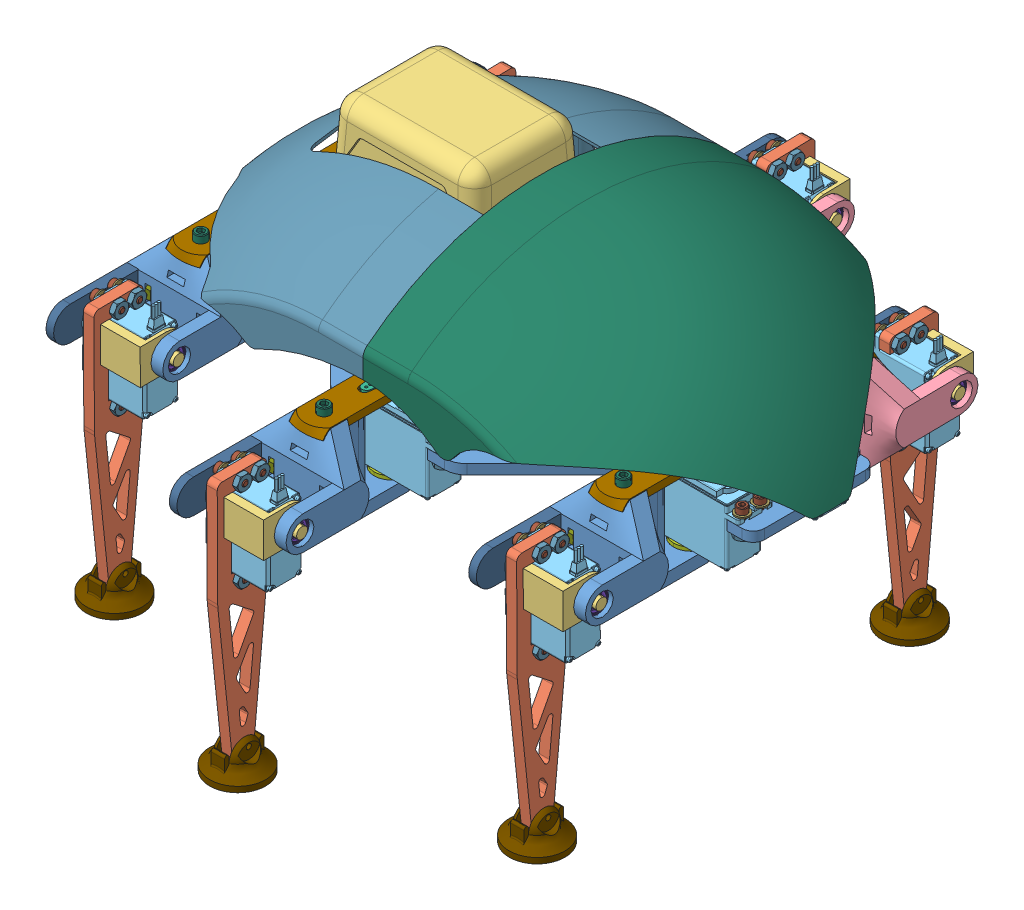
SolidWorks assembly Hexapod_(Leg_V1+Body_V2), configuration Défaut. Lengths in mm.
Overall size (338.69 233.7 350.76).
398 component instances, 33 part files, 150 mates.
Components (placement in the parent):
- Body_V2-5: Body_V2 [Default] at (-310 -5.6 15) x (1 0 0) z (0 1 0) size (310 170 5.6)
- Leg_(Straight_Foot)-6: Leg_(Straight_Foot) [Default] at (-54.94 -26.67 -0.094) size (71.12 162.26 125.96)
  - Foot_(Straight)-1: Foot_(Straight) [Default] at (4.9357 4.6699 -91.3683) x (0.014203 -0.004158 0.99989) z (-0.999899 0 0.014203) size (28 145.4 6)
  - bearing_mount_foot-1: bearing_mount_foot [Default] at (4.8169 16.6428 -99.7277) x (-0.014203 0.004158 -0.99989) z (0.999899 0 -0.014203) size (25 20 29.5)
  - Joint-1: Joint [Défaut] at (35.768 26.4662 -54.7315) x (-0.014203 0 -0.999899) z (0 1 0) size (96.52 53.26 53.26)
  - hs-422-2: hs-422 [Défaut] at (5.1023 6.6131 -77.4551) x (-0.014203 0.004158 -0.99989) z (0.000059 0.999991 0.004158) size (19.81 42.09 58.23)
  - hs-422-3: hs-422 [Défaut] at (19.939 20.701 -19.812) x (0 0 1) z (-1 0 0) size (19.81 42.09 58.23)
  - hs-422_horn_straight-1: hs-422_horn_straight [Default] at (-16.9088 16.9412 -87.0065) x (0.014203 0 0.999899) z (0 1 0) size (33.93 4.93 8.79)
  - hs-422_horn_straight-2: hs-422_horn_straight [Default] at (9.652 42.5743 -9.906) x (-0.014203 0 -0.999899) z (-0.999899 0 0.014203) size (33.93 4.93 8.79)
  - Bearing_mount_leg-1: Bearing_mount_leg [Default] at (9.652 21 2.594) x (0 0 1) z (0 -1 0) size (35 20 30)
  - Bearing-1: Bearing [Default] at (9.652 -6.7498 -9.906) x (0.84763 0 0.530588) z (-0.530588 0 0.84763) size (13.87 4.75 13.87)
  - Bearing-2: Bearing [Default] at (32.2403 16.9412 -87.7047) x (0.007588 -0.845349 0.534161) z (-0.012007 -0.534214 -0.845264) size (13.87 4.75 13.87)
  - Joint_attachment_leg-1: Joint_attachment_leg [Défaut] at (35.768 26.4662 -54.7315) x (-0.014203 0 -0.999899) z (0 1 0) size (74.32 19.07 4.32)
  - Joint_attachment_foot-1: Joint_attachment_foot [Défaut] at (35.768 26.4662 -54.7315) x (-0.014203 0 -0.999899) z (0 1 0) size (64.08 6.7 19.07)
  - socket_1_2_6-32_with_washer-1: socket_1_2_6-32_with_washer [Défaut] at (43.4196 -14.698 -83.8589) x (0.999899 0 -0.014203) z (0.012271 -0.503597 0.863852) size (16.21 7.92 7.92)
    - HX-SHCS 0.138-32x0.5x0.5-N-1: HX-SHCS 0.138-32x0.5x0.5-N [HX-SHCS 0.138-32x0.5x0.5-N] at (-51.206 -1.62 2.0257) size (16.21 5.74 5.74)
    - Narrow FW 0.138-1: Narrow FW 0.138 [Narrow FW 0.138] at (-46.888 -1.62 2.0257) size (0.81 7.92 7.92)
  - socket_1_2_6-32_with_washer-2: socket_1_2_6-32_with_washer [Défaut] at (43.2654 -19.0943 -94.7118) x (0.999899 0 -0.014203) z (0.000059 0.999991 0.004158) size (16.21 7.92 7.92)
    - HX-SHCS 0.138-32x0.5x0.5-N-1: HX-SHCS 0.138-32x0.5x0.5-N [HX-SHCS 0.138-32x0.5x0.5-N] at (-51.206 -1.62 2.0257) size (16.21 5.74 5.74)
    - Narrow FW 0.138-1: Narrow FW 0.138 [Narrow FW 0.138] at (-46.888 -1.62 2.0257) size (0.81 7.92 7.92)
  - socket_1_2_6-32_with_washer-3: socket_1_2_6-32_with_washer [Défaut] at (43.4489 27.9623 -81.7931) x (0.999899 0 -0.014203) z (-0.012271 0.503597 -0.863852) size (16.21 7.92 7.92)
    - HX-SHCS 0.138-32x0.5x0.5-N-1: HX-SHCS 0.138-32x0.5x0.5-N [HX-SHCS 0.138-32x0.5x0.5-N] at (-51.206 -1.62 2.0257) size (16.21 5.74 5.74)
    - Narrow FW 0.138-1: Narrow FW 0.138 [Narrow FW 0.138] at (-46.888 -1.62 2.0257) size (0.81 7.92 7.92)
  - socket_1_2_6-32_with_washer-4: socket_1_2_6-32_with_washer [Défaut] at (43.3046 28.0045 -91.952) x (0.999899 0 -0.014203) z (-0.012271 0.503597 -0.863852) size (16.21 7.92 7.92)
    - HX-SHCS 0.138-32x0.5x0.5-N-1: HX-SHCS 0.138-32x0.5x0.5-N [HX-SHCS 0.138-32x0.5x0.5-N] at (-51.206 -1.62 2.0257) size (16.21 5.74 5.74)
    - Narrow FW 0.138-1: Narrow FW 0.138 [Narrow FW 0.138] at (-46.888 -1.62 2.0257) size (0.81 7.92 7.92)
  - SBHCSCREW 0.112-40x0.25-HX-N-2: SBHCSCREW 0.112-40x0.25-HX-N [SBHCSCREW 0.112-40x0.25-HX-N] at (-19.9057 16.9412 -86.964) x (0.999899 0 -0.014203) z (-0.007102 0.866025 -0.49995) size (7.85 5.41 5.41)
  - SBHCSCREW 0.112-40x0.25-HX-N-3: SBHCSCREW 0.112-40x0.25-HX-N [SBHCSCREW 0.112-40x0.25-HX-N] at (9.652 45.5715 -9.906) x (0 -1 0) z (0.87304 0 0.487649) size (7.85 5.41 5.41)
  - MSHXNUT 0.138-32-D-N-11: MSHXNUT 0.138-32-D-N [MSHXNUT 0.138-32-D-N] at (5.0634 -17.1176 -82.3797) x (0.01233 0.496395 0.868009) z (-0.999899 0 0.014203) size (7.92 9.15 2.9)
  - MSHXNUT 0.138-32-D-N-12: MSHXNUT 0.138-32-D-N [MSHXNUT 0.138-32-D-N] at (4.9191 -17.0754 -92.5386) x (-0.012271 0.503597 -0.863852) z (-0.999899 0 0.014203) size (7.92 9.15 2.9)
  - MSHXNUT 0.138-32-D-N-13: MSHXNUT 0.138-32-D-N [MSHXNUT 0.138-32-D-N] at (5.0662 30.382 -82.1822) x (0.000059 0.999991 0.004158) z (-0.999899 0 0.014203) size (7.92 9.15 2.9)
  - MSHXNUT 0.138-32-D-N-14: MSHXNUT 0.138-32-D-N [MSHXNUT 0.138-32-D-N] at (4.9219 30.4242 -92.3411) x (0.000059 0.999991 0.004158) z (-0.999899 0 0.014203) size (7.92 9.15 2.9)
  - HX-SHCS 0.164-32x0.5x0.5-N-1: HX-SHCS 0.164-32x0.5x0.5-N [HX-SHCS 0.164-32x0.5x0.5-N] at (9.1052 47.8568 -48.4) x (0 -1 0) z (0.014203 0 0.999899) size (16.87 6.86 6.86)
  - HX-SHCS 0.164-32x0.5x0.5-N-2: HX-SHCS 0.164-32x0.5x0.5-N [HX-SHCS 0.164-32x0.5x0.5-N] at (-21.967 16.9412 -59.205) x (0.999899 0 -0.014203) z (0.014203 0 0.999899) size (16.87 6.86 6.86)
  - MSHXNUT 0.164-32-D-N-11: MSHXNUT 0.164-32-D-N [MSHXNUT 0.164-32-D-N] at (9.1052 33.127 -48.4) x (0.87304 0 0.487649) z (0 1 0) size (8.74 10.09 3.3)
  - MSHXNUT 0.164-32-D-N-12: MSHXNUT 0.164-32-D-N [MSHXNUT 0.164-32-D-N] at (-7.2387 16.9412 -59.4142) x (0.014203 0 0.999899) z (-0.999899 0 0.014203) size (8.74 10.09 3.3)
  - HX-SHCS 0.112-40x0.5x0.5-N-5: HX-SHCS 0.112-40x0.5x0.5-N [HX-SHCS 0.112-40x0.5x0.5-N] at (-4.0273 11.7048 -99.6226) x (0.999899 0 -0.014203) z (0.014203 -0.004158 0.99989) size (15.54 4.65 4.65)
  - HX-SHCS 0.112-40x0.5x0.5-N-6: HX-SHCS 0.112-40x0.5x0.5-N [HX-SHCS 0.112-40x0.5x0.5-N] at (-4.0267 21.7048 -99.5811) x (0.999899 0 -0.014203) z (-0.014203 0.004158 -0.99989) size (15.54 4.65 4.65)
  - socket_1_2_6-32_with_washer-5: socket_1_2_6-32_with_washer [Défaut] at (-3.4199 -17.7034 -7.3903) x (0 -1 0) z (0.5 0 0.866025) size (16.21 7.92 7.92)
    - HX-SHCS 0.138-32x0.5x0.5-N-1: HX-SHCS 0.138-32x0.5x0.5-N [HX-SHCS 0.138-32x0.5x0.5-N] at (-51.206 -1.62 2.0257) size (16.21 5.74 5.74)
    - Narrow FW 0.138-1: Narrow FW 0.138 [Narrow FW 0.138] at (-46.888 -1.62 2.0257) size (0.81 7.92 7.92)
  - socket_1_2_6-32_with_washer-6: socket_1_2_6-32_with_washer [Défaut] at (44.0781 -17.7034 -17.5503) x (0 -1 0) z (0.5 0 0.866025) size (16.21 7.92 7.92)
    - HX-SHCS 0.138-32x0.5x0.5-N-1: HX-SHCS 0.138-32x0.5x0.5-N [HX-SHCS 0.138-32x0.5x0.5-N] at (-51.206 -1.62 2.0257) size (16.21 5.74 5.74)
    - Narrow FW 0.138-1: Narrow FW 0.138 [Narrow FW 0.138] at (-46.888 -1.62 2.0257) size (0.81 7.92 7.92)
  - socket_1_2_6-32_with_washer-7: socket_1_2_6-32_with_washer [Défaut] at (-3.4199 -17.7034 -17.5503) x (0 -1 0) z (0.5 0 0.866025) size (16.21 7.92 7.92)
    - HX-SHCS 0.138-32x0.5x0.5-N-1: HX-SHCS 0.138-32x0.5x0.5-N [HX-SHCS 0.138-32x0.5x0.5-N] at (-51.206 -1.62 2.0257) size (16.21 5.74 5.74)
    - Narrow FW 0.138-1: Narrow FW 0.138 [Narrow FW 0.138] at (-46.888 -1.62 2.0257) size (0.81 7.92 7.92)
  - socket_1_2_6-32_with_washer-8: socket_1_2_6-32_with_washer [Défaut] at (44.0781 -17.7034 -7.3903) x (0 -1 0) z (0.5 0 0.866025) size (16.21 7.92 7.92)
    - HX-SHCS 0.138-32x0.5x0.5-N-1: HX-SHCS 0.138-32x0.5x0.5-N [HX-SHCS 0.138-32x0.5x0.5-N] at (-51.206 -1.62 2.0257) size (16.21 5.74 5.74)
    - Narrow FW 0.138-1: Narrow FW 0.138 [Narrow FW 0.138] at (-46.888 -1.62 2.0257) size (0.81 7.92 7.92)
  - Slippers-1: Slippers [Default] at (1.9298 -111.2299 -91.7597) x (0.999899 0 -0.014203) z (0.014203 0 0.999899) size (35.48 18.25 37.71)
- Leg_(Straight_Foot)-7: Leg_(Straight_Foot) [Default] at (-294.94 -26.67 -0.094) size (71.12 162.26 125.96)
  - Foot_(Straight)-1: Foot_(Straight) [Default] at (4.9357 4.6699 -91.3683) x (0.014203 -0.004158 0.99989) z (-0.999899 0 0.014203) size (28 145.4 6)
  - bearing_mount_foot-1: bearing_mount_foot [Default] at (4.8169 16.6428 -99.7277) x (-0.014203 0.004158 -0.99989) z (0.999899 0 -0.014203) size (25 20 29.5)
  - Joint-1: Joint [Défaut] at (35.768 26.4662 -54.7315) x (-0.014203 0 -0.999899) z (0 1 0) size (96.52 53.26 53.26)
  - hs-422-2: hs-422 [Défaut] at (5.1023 6.6131 -77.4551) x (-0.014203 0.004158 -0.99989) z (0.000059 0.999991 0.004158) size (19.81 42.09 58.23)
  - hs-422-3: hs-422 [Défaut] at (19.939 20.701 -19.812) x (0 0 1) z (-1 0 0) size (19.81 42.09 58.23)
  - hs-422_horn_straight-1: hs-422_horn_straight [Default] at (-16.9088 16.9412 -87.0065) x (0.014203 0 0.999899) z (0 1 0) size (33.93 4.93 8.79)
  - hs-422_horn_straight-2: hs-422_horn_straight [Default] at (9.652 42.5743 -9.906) x (-0.014203 0 -0.999899) z (-0.999899 0 0.014203) size (33.93 4.93 8.79)
  - Bearing_mount_leg-1: Bearing_mount_leg [Default] at (9.652 21 2.594) x (0 0 1) z (0 -1 0) size (35 20 30)
  - Bearing-1: Bearing [Default] at (9.652 -6.7498 -9.906) x (0.84763 0 0.530588) z (-0.530588 0 0.84763) size (13.87 4.75 13.87)
  - Bearing-2: Bearing [Default] at (32.2403 16.9412 -87.7047) x (0.007588 -0.845349 0.534161) z (-0.012007 -0.534214 -0.845264) size (13.87 4.75 13.87)
  - Joint_attachment_leg-1: Joint_attachment_leg [Défaut] at (35.768 26.4662 -54.7315) x (-0.014203 0 -0.999899) z (0 1 0) size (74.32 19.07 4.32)
  - Joint_attachment_foot-1: Joint_attachment_foot [Défaut] at (35.768 26.4662 -54.7315) x (-0.014203 0 -0.999899) z (0 1 0) size (64.08 6.7 19.07)
  - socket_1_2_6-32_with_washer-1: socket_1_2_6-32_with_washer [Défaut] at (43.4196 -14.698 -83.8589) x (0.999899 0 -0.014203) z (0.012271 -0.503597 0.863852) size (16.21 7.92 7.92)
    - HX-SHCS 0.138-32x0.5x0.5-N-1: HX-SHCS 0.138-32x0.5x0.5-N [HX-SHCS 0.138-32x0.5x0.5-N] at (-51.206 -1.62 2.0257) size (16.21 5.74 5.74)
    - Narrow FW 0.138-1: Narrow FW 0.138 [Narrow FW 0.138] at (-46.888 -1.62 2.0257) size (0.81 7.92 7.92)
  - socket_1_2_6-32_with_washer-2: socket_1_2_6-32_with_washer [Défaut] at (43.2654 -19.0943 -94.7118) x (0.999899 0 -0.014203) z (0.000059 0.999991 0.004158) size (16.21 7.92 7.92)
    - HX-SHCS 0.138-32x0.5x0.5-N-1: HX-SHCS 0.138-32x0.5x0.5-N [HX-SHCS 0.138-32x0.5x0.5-N] at (-51.206 -1.62 2.0257) size (16.21 5.74 5.74)
    - Narrow FW 0.138-1: Narrow FW 0.138 [Narrow FW 0.138] at (-46.888 -1.62 2.0257) size (0.81 7.92 7.92)
  - socket_1_2_6-32_with_washer-3: socket_1_2_6-32_with_washer [Défaut] at (43.4489 27.9623 -81.7931) x (0.999899 0 -0.014203) z (-0.012271 0.503597 -0.863852) size (16.21 7.92 7.92)
    - HX-SHCS 0.138-32x0.5x0.5-N-1: HX-SHCS 0.138-32x0.5x0.5-N [HX-SHCS 0.138-32x0.5x0.5-N] at (-51.206 -1.62 2.0257) size (16.21 5.74 5.74)
    - Narrow FW 0.138-1: Narrow FW 0.138 [Narrow FW 0.138] at (-46.888 -1.62 2.0257) size (0.81 7.92 7.92)
  - socket_1_2_6-32_with_washer-4: socket_1_2_6-32_with_washer [Défaut] at (43.3046 28.0045 -91.952) x (0.999899 0 -0.014203) z (-0.012271 0.503597 -0.863852) size (16.21 7.92 7.92)
    - HX-SHCS 0.138-32x0.5x0.5-N-1: HX-SHCS 0.138-32x0.5x0.5-N [HX-SHCS 0.138-32x0.5x0.5-N] at (-51.206 -1.62 2.0257) size (16.21 5.74 5.74)
    - Narrow FW 0.138-1: Narrow FW 0.138 [Narrow FW 0.138] at (-46.888 -1.62 2.0257) size (0.81 7.92 7.92)
  - SBHCSCREW 0.112-40x0.25-HX-N-2: SBHCSCREW 0.112-40x0.25-HX-N [SBHCSCREW 0.112-40x0.25-HX-N] at (-19.9057 16.9412 -86.964) x (0.999899 0 -0.014203) z (-0.007102 0.866025 -0.49995) size (7.85 5.41 5.41)
  - SBHCSCREW 0.112-40x0.25-HX-N-3: SBHCSCREW 0.112-40x0.25-HX-N [SBHCSCREW 0.112-40x0.25-HX-N] at (9.652 45.5715 -9.906) x (0 -1 0) z (0.87304 0 0.487649) size (7.85 5.41 5.41)
  - MSHXNUT 0.138-32-D-N-11: MSHXNUT 0.138-32-D-N [MSHXNUT 0.138-32-D-N] at (5.0634 -17.1176 -82.3797) x (0.01233 0.496395 0.868009) z (-0.999899 0 0.014203) size (7.92 9.15 2.9)
  - MSHXNUT 0.138-32-D-N-12: MSHXNUT 0.138-32-D-N [MSHXNUT 0.138-32-D-N] at (4.9191 -17.0754 -92.5386) x (-0.012271 0.503597 -0.863852) z (-0.999899 0 0.014203) size (7.92 9.15 2.9)
  - MSHXNUT 0.138-32-D-N-13: MSHXNUT 0.138-32-D-N [MSHXNUT 0.138-32-D-N] at (5.0662 30.382 -82.1822) x (0.000059 0.999991 0.004158) z (-0.999899 0 0.014203) size (7.92 9.15 2.9)
  - MSHXNUT 0.138-32-D-N-14: MSHXNUT 0.138-32-D-N [MSHXNUT 0.138-32-D-N] at (4.9219 30.4242 -92.3411) x (0.000059 0.999991 0.004158) z (-0.999899 0 0.014203) size (7.92 9.15 2.9)
  - HX-SHCS 0.164-32x0.5x0.5-N-1: HX-SHCS 0.164-32x0.5x0.5-N [HX-SHCS 0.164-32x0.5x0.5-N] at (9.1052 47.8568 -48.4) x (0 -1 0) z (0.014203 0 0.999899) size (16.87 6.86 6.86)
  - HX-SHCS 0.164-32x0.5x0.5-N-2: HX-SHCS 0.164-32x0.5x0.5-N [HX-SHCS 0.164-32x0.5x0.5-N] at (-21.967 16.9412 -59.205) x (0.999899 0 -0.014203) z (0.014203 0 0.999899) size (16.87 6.86 6.86)
  - MSHXNUT 0.164-32-D-N-11: MSHXNUT 0.164-32-D-N [MSHXNUT 0.164-32-D-N] at (9.1052 33.127 -48.4) x (0.87304 0 0.487649) z (0 1 0) size (8.74 10.09 3.3)
  - MSHXNUT 0.164-32-D-N-12: MSHXNUT 0.164-32-D-N [MSHXNUT 0.164-32-D-N] at (-7.2387 16.9412 -59.4142) x (0.014203 0 0.999899) z (-0.999899 0 0.014203) size (8.74 10.09 3.3)
  - HX-SHCS 0.112-40x0.5x0.5-N-5: HX-SHCS 0.112-40x0.5x0.5-N [HX-SHCS 0.112-40x0.5x0.5-N] at (-4.0273 11.7048 -99.6226) x (0.999899 0 -0.014203) z (0.014203 -0.004158 0.99989) size (15.54 4.65 4.65)
  - HX-SHCS 0.112-40x0.5x0.5-N-6: HX-SHCS 0.112-40x0.5x0.5-N [HX-SHCS 0.112-40x0.5x0.5-N] at (-4.0267 21.7048 -99.5811) x (0.999899 0 -0.014203) z (-0.014203 0.004158 -0.99989) size (15.54 4.65 4.65)
  - socket_1_2_6-32_with_washer-5: socket_1_2_6-32_with_washer [Défaut] at (-3.4199 -17.7034 -7.3903) x (0 -1 0) z (0.5 0 0.866025) size (16.21 7.92 7.92)
    - HX-SHCS 0.138-32x0.5x0.5-N-1: HX-SHCS 0.138-32x0.5x0.5-N [HX-SHCS 0.138-32x0.5x0.5-N] at (-51.206 -1.62 2.0257) size (16.21 5.74 5.74)
    - Narrow FW 0.138-1: Narrow FW 0.138 [Narrow FW 0.138] at (-46.888 -1.62 2.0257) size (0.81 7.92 7.92)
  - socket_1_2_6-32_with_washer-6: socket_1_2_6-32_with_washer [Défaut] at (44.0781 -17.7034 -17.5503) x (0 -1 0) z (0.5 0 0.866025) size (16.21 7.92 7.92)
    - HX-SHCS 0.138-32x0.5x0.5-N-1: HX-SHCS 0.138-32x0.5x0.5-N [HX-SHCS 0.138-32x0.5x0.5-N] at (-51.206 -1.62 2.0257) size (16.21 5.74 5.74)
    - Narrow FW 0.138-1: Narrow FW 0.138 [Narrow FW 0.138] at (-46.888 -1.62 2.0257) size (0.81 7.92 7.92)
  - socket_1_2_6-32_with_washer-7: socket_1_2_6-32_with_washer [Défaut] at (-3.4199 -17.7034 -17.5503) x (0 -1 0) z (0.5 0 0.866025) size (16.21 7.92 7.92)
    - HX-SHCS 0.138-32x0.5x0.5-N-1: HX-SHCS 0.138-32x0.5x0.5-N [HX-SHCS 0.138-32x0.5x0.5-N] at (-51.206 -1.62 2.0257) size (16.21 5.74 5.74)
    - Narrow FW 0.138-1: Narrow FW 0.138 [Narrow FW 0.138] at (-46.888 -1.62 2.0257) size (0.81 7.92 7.92)
  - socket_1_2_6-32_with_washer-8: socket_1_2_6-32_with_washer [Défaut] at (44.0781 -17.7034 -7.3903) x (0 -1 0) z (0.5 0 0.866025) size (16.21 7.92 7.92)
    - HX-SHCS 0.138-32x0.5x0.5-N-1: HX-SHCS 0.138-32x0.5x0.5-N [HX-SHCS 0.138-32x0.5x0.5-N] at (-51.206 -1.62 2.0257) size (16.21 5.74 5.74)
    - Narrow FW 0.138-1: Narrow FW 0.138 [Narrow FW 0.138] at (-46.888 -1.62 2.0257) size (0.81 7.92 7.92)
  - Slippers-1: Slippers [Default] at (1.9298 -111.2299 -91.7597) x (0.999899 0 -0.014203) z (0.014203 0 0.999899) size (35.48 18.25 37.71)
- Leg_(Straight_Foot)-8: Leg_(Straight_Foot) [Default] at (-174.94 -26.67 -50.094) size (71.12 162.26 125.96)
  - Foot_(Straight)-1: Foot_(Straight) [Default] at (4.9357 4.6699 -91.3683) x (0.014203 -0.004158 0.99989) z (-0.999899 0 0.014203) size (28 145.4 6)
  - bearing_mount_foot-1: bearing_mount_foot [Default] at (4.8169 16.6428 -99.7277) x (-0.014203 0.004158 -0.99989) z (0.999899 0 -0.014203) size (25 20 29.5)
  - Joint-1: Joint [Défaut] at (35.768 26.4662 -54.7315) x (-0.014203 0 -0.999899) z (0 1 0) size (96.52 53.26 53.26)
  - hs-422-2: hs-422 [Défaut] at (5.1023 6.6131 -77.4551) x (-0.014203 0.004158 -0.99989) z (0.000059 0.999991 0.004158) size (19.81 42.09 58.23)
  - hs-422-3: hs-422 [Défaut] at (19.939 20.701 -19.812) x (0 0 1) z (-1 0 0) size (19.81 42.09 58.23)
  - hs-422_horn_straight-1: hs-422_horn_straight [Default] at (-16.9088 16.9412 -87.0065) x (0.014203 0 0.999899) z (0 1 0) size (33.93 4.93 8.79)
  - hs-422_horn_straight-2: hs-422_horn_straight [Default] at (9.652 42.5743 -9.906) x (-0.014203 0 -0.999899) z (-0.999899 0 0.014203) size (33.93 4.93 8.79)
  - Bearing_mount_leg-1: Bearing_mount_leg [Default] at (9.652 21 2.594) x (0 0 1) z (0 -1 0) size (35 20 30)
  - Bearing-1: Bearing [Default] at (9.652 -6.7498 -9.906) x (0.84763 0 0.530588) z (-0.530588 0 0.84763) size (13.87 4.75 13.87)
  - Bearing-2: Bearing [Default] at (32.2403 16.9412 -87.7047) x (0.007588 -0.845349 0.534161) z (-0.012007 -0.534214 -0.845264) size (13.87 4.75 13.87)
  - Joint_attachment_leg-1: Joint_attachment_leg [Défaut] at (35.768 26.4662 -54.7315) x (-0.014203 0 -0.999899) z (0 1 0) size (74.32 19.07 4.32)
  - Joint_attachment_foot-1: Joint_attachment_foot [Défaut] at (35.768 26.4662 -54.7315) x (-0.014203 0 -0.999899) z (0 1 0) size (64.08 6.7 19.07)
  - socket_1_2_6-32_with_washer-1: socket_1_2_6-32_with_washer [Défaut] at (43.4196 -14.698 -83.8589) x (0.999899 0 -0.014203) z (0.012271 -0.503597 0.863852) size (16.21 7.92 7.92)
    - HX-SHCS 0.138-32x0.5x0.5-N-1: HX-SHCS 0.138-32x0.5x0.5-N [HX-SHCS 0.138-32x0.5x0.5-N] at (-51.206 -1.62 2.0257) size (16.21 5.74 5.74)
    - Narrow FW 0.138-1: Narrow FW 0.138 [Narrow FW 0.138] at (-46.888 -1.62 2.0257) size (0.81 7.92 7.92)
  - socket_1_2_6-32_with_washer-2: socket_1_2_6-32_with_washer [Défaut] at (43.2654 -19.0943 -94.7118) x (0.999899 0 -0.014203) z (0.000059 0.999991 0.004158) size (16.21 7.92 7.92)
    - HX-SHCS 0.138-32x0.5x0.5-N-1: HX-SHCS 0.138-32x0.5x0.5-N [HX-SHCS 0.138-32x0.5x0.5-N] at (-51.206 -1.62 2.0257) size (16.21 5.74 5.74)
    - Narrow FW 0.138-1: Narrow FW 0.138 [Narrow FW 0.138] at (-46.888 -1.62 2.0257) size (0.81 7.92 7.92)
  - socket_1_2_6-32_with_washer-3: socket_1_2_6-32_with_washer [Défaut] at (43.4489 27.9623 -81.7931) x (0.999899 0 -0.014203) z (-0.012271 0.503597 -0.863852) size (16.21 7.92 7.92)
    - HX-SHCS 0.138-32x0.5x0.5-N-1: HX-SHCS 0.138-32x0.5x0.5-N [HX-SHCS 0.138-32x0.5x0.5-N] at (-51.206 -1.62 2.0257) size (16.21 5.74 5.74)
    - Narrow FW 0.138-1: Narrow FW 0.138 [Narrow FW 0.138] at (-46.888 -1.62 2.0257) size (0.81 7.92 7.92)
  - socket_1_2_6-32_with_washer-4: socket_1_2_6-32_with_washer [Défaut] at (43.3046 28.0045 -91.952) x (0.999899 0 -0.014203) z (-0.012271 0.503597 -0.863852) size (16.21 7.92 7.92)
    - HX-SHCS 0.138-32x0.5x0.5-N-1: HX-SHCS 0.138-32x0.5x0.5-N [HX-SHCS 0.138-32x0.5x0.5-N] at (-51.206 -1.62 2.0257) size (16.21 5.74 5.74)
    - Narrow FW 0.138-1: Narrow FW 0.138 [Narrow FW 0.138] at (-46.888 -1.62 2.0257) size (0.81 7.92 7.92)
  - SBHCSCREW 0.112-40x0.25-HX-N-2: SBHCSCREW 0.112-40x0.25-HX-N [SBHCSCREW 0.112-40x0.25-HX-N] at (-19.9057 16.9412 -86.964) x (0.999899 0 -0.014203) z (-0.007102 0.866025 -0.49995) size (7.85 5.41 5.41)
  - SBHCSCREW 0.112-40x0.25-HX-N-3: SBHCSCREW 0.112-40x0.25-HX-N [SBHCSCREW 0.112-40x0.25-HX-N] at (9.652 45.5715 -9.906) x (0 -1 0) z (0.87304 0 0.487649) size (7.85 5.41 5.41)
  - MSHXNUT 0.138-32-D-N-11: MSHXNUT 0.138-32-D-N [MSHXNUT 0.138-32-D-N] at (5.0634 -17.1176 -82.3797) x (0.01233 0.496395 0.868009) z (-0.999899 0 0.014203) size (7.92 9.15 2.9)
  - MSHXNUT 0.138-32-D-N-12: MSHXNUT 0.138-32-D-N [MSHXNUT 0.138-32-D-N] at (4.9191 -17.0754 -92.5386) x (-0.012271 0.503597 -0.863852) z (-0.999899 0 0.014203) size (7.92 9.15 2.9)
  - MSHXNUT 0.138-32-D-N-13: MSHXNUT 0.138-32-D-N [MSHXNUT 0.138-32-D-N] at (5.0662 30.382 -82.1822) x (0.000059 0.999991 0.004158) z (-0.999899 0 0.014203) size (7.92 9.15 2.9)
  - MSHXNUT 0.138-32-D-N-14: MSHXNUT 0.138-32-D-N [MSHXNUT 0.138-32-D-N] at (4.9219 30.4242 -92.3411) x (0.000059 0.999991 0.004158) z (-0.999899 0 0.014203) size (7.92 9.15 2.9)
  - HX-SHCS 0.164-32x0.5x0.5-N-1: HX-SHCS 0.164-32x0.5x0.5-N [HX-SHCS 0.164-32x0.5x0.5-N] at (9.1052 47.8568 -48.4) x (0 -1 0) z (0.014203 0 0.999899) size (16.87 6.86 6.86)
  - HX-SHCS 0.164-32x0.5x0.5-N-2: HX-SHCS 0.164-32x0.5x0.5-N [HX-SHCS 0.164-32x0.5x0.5-N] at (-21.967 16.9412 -59.205) x (0.999899 0 -0.014203) z (0.014203 0 0.999899) size (16.87 6.86 6.86)
  - MSHXNUT 0.164-32-D-N-11: MSHXNUT 0.164-32-D-N [MSHXNUT 0.164-32-D-N] at (9.1052 33.127 -48.4) x (0.87304 0 0.487649) z (0 1 0) size (8.74 10.09 3.3)
  - MSHXNUT 0.164-32-D-N-12: MSHXNUT 0.164-32-D-N [MSHXNUT 0.164-32-D-N] at (-7.2387 16.9412 -59.4142) x (0.014203 0 0.999899) z (-0.999899 0 0.014203) size (8.74 10.09 3.3)
  - HX-SHCS 0.112-40x0.5x0.5-N-5: HX-SHCS 0.112-40x0.5x0.5-N [HX-SHCS 0.112-40x0.5x0.5-N] at (-4.0273 11.7048 -99.6226) x (0.999899 0 -0.014203) z (0.014203 -0.004158 0.99989) size (15.54 4.65 4.65)
  - HX-SHCS 0.112-40x0.5x0.5-N-6: HX-SHCS 0.112-40x0.5x0.5-N [HX-SHCS 0.112-40x0.5x0.5-N] at (-4.0267 21.7048 -99.5811) x (0.999899 0 -0.014203) z (-0.014203 0.004158 -0.99989) size (15.54 4.65 4.65)
  - socket_1_2_6-32_with_washer-5: socket_1_2_6-32_with_washer [Défaut] at (-3.4199 -17.7034 -7.3903) x (0 -1 0) z (0.5 0 0.866025) size (16.21 7.92 7.92)
    - HX-SHCS 0.138-32x0.5x0.5-N-1: HX-SHCS 0.138-32x0.5x0.5-N [HX-SHCS 0.138-32x0.5x0.5-N] at (-51.206 -1.62 2.0257) size (16.21 5.74 5.74)
    - Narrow FW 0.138-1: Narrow FW 0.138 [Narrow FW 0.138] at (-46.888 -1.62 2.0257) size (0.81 7.92 7.92)
  - socket_1_2_6-32_with_washer-6: socket_1_2_6-32_with_washer [Défaut] at (44.0781 -17.7034 -17.5503) x (0 -1 0) z (0.5 0 0.866025) size (16.21 7.92 7.92)
    - HX-SHCS 0.138-32x0.5x0.5-N-1: HX-SHCS 0.138-32x0.5x0.5-N [HX-SHCS 0.138-32x0.5x0.5-N] at (-51.206 -1.62 2.0257) size (16.21 5.74 5.74)
    - Narrow FW 0.138-1: Narrow FW 0.138 [Narrow FW 0.138] at (-46.888 -1.62 2.0257) size (0.81 7.92 7.92)
  - socket_1_2_6-32_with_washer-7: socket_1_2_6-32_with_washer [Défaut] at (-3.4199 -17.7034 -17.5503) x (0 -1 0) z (0.5 0 0.866025) size (16.21 7.92 7.92)
    - HX-SHCS 0.138-32x0.5x0.5-N-1: HX-SHCS 0.138-32x0.5x0.5-N [HX-SHCS 0.138-32x0.5x0.5-N] at (-51.206 -1.62 2.0257) size (16.21 5.74 5.74)
    - Narrow FW 0.138-1: Narrow FW 0.138 [Narrow FW 0.138] at (-46.888 -1.62 2.0257) size (0.81 7.92 7.92)
  - socket_1_2_6-32_with_washer-8: socket_1_2_6-32_with_washer [Défaut] at (44.0781 -17.7034 -7.3903) x (0 -1 0) z (0.5 0 0.866025) size (16.21 7.92 7.92)
    - HX-SHCS 0.138-32x0.5x0.5-N-1: HX-SHCS 0.138-32x0.5x0.5-N [HX-SHCS 0.138-32x0.5x0.5-N] at (-51.206 -1.62 2.0257) size (16.21 5.74 5.74)
    - Narrow FW 0.138-1: Narrow FW 0.138 [Narrow FW 0.138] at (-46.888 -1.62 2.0257) size (0.81 7.92 7.92)
  - Slippers-1: Slippers [Default] at (1.9298 -111.2299 -91.7597) x (0.999899 0 -0.014203) z (0.014203 0 0.999899) size (35.48 18.25 37.71)
- Leg_(Straight_Foot)_(Mirror)-4: Leg_(Straight_Foot)_(Mirror) [Default] at (-294.94 -26.67 49.906) size (70.34 162.3 124.8)
  - Joint_(Mirror)-1: Joint_(Mirror) [Défaut] at (36.4933 -51.1276 34.4889) x (0.002055 0 0.999998) z (0 -1 0) size (96.52 53.26 53.26)
  - hs-422-3: hs-422 [Défaut] at (19.939 20.701 -19.812) x (0 0 1) z (-1 0 0) size (19.81 42.09 58.23)
  - hs-422_horn_straight-2: hs-422_horn_straight [Default] at (9.652 42.5743 -9.906) x (0.002055 0 0.999998) z (0.999998 0 -0.002055) size (33.93 4.93 8.79)
  - Bearing_mount_leg-1: Bearing_mount_leg [Default] at (9.652 21 -22.406) x (0 0 -1) z (0 -1 0) size (35 20 30)
  - Bearing-1: Bearing [Default] at (9.652 -6.7498 -9.906) x (0.266287 0 0.963894) z (-0.963894 0 0.266287) size (13.87 4.75 13.87)
  - Joint_attachment_leg-1: Joint_attachment_leg [Défaut] at (-17.0066 26.5024 34.5989) x (0.002055 0 0.999998) z (0 1 0) size (74.32 19.07 4.32)
  - bearing_mount_foot-2: bearing_mount_foot [Default] at (6.7141 17.2663 79.9818) x (0.002055 -0.004919 0.999986) z (0.999998 0 -0.002055) size (25 20 29.5)
  - Bearing-3: Bearing [Default] at (29.1886 16.9774 67.524) x (-0.001098 -0.845349 -0.534213) z (0.001738 -0.534214 0.845347) size (13.87 4.75 13.87)
  - hs-422-4: hs-422 [Défaut] at (6.0779 6.6418 77.4268) x (-0.002055 0.004919 -0.999986) z (0.00001 0.999988 0.004919) size (19.81 42.09 58.23)
  - hs-422_horn_straight-3: hs-422_horn_straight [Default] at (-15.8156 16.9774 67.6165) x (-0.002055 0 -0.999998) z (0 -1 0) size (33.93 4.93 8.79)
  - Foot_(Straight)-2: Foot_(Straight) [Default] at (0.0967 4.6719 71.5233) x (-0.002055 0.004919 -0.999986) z (0.999998 0 -0.002055) size (28 145.4 6)
  - Joint_attachment_foot-2: Joint_attachment_foot [Défaut] at (36.4933 7.4524 34.4889) x (0.002055 0 0.999998) z (0 -1 0) size (64.08 6.7 19.07)
  - SBHCSCREW 0.138-32x0.25-HX-N-1: SBHCSCREW 0.138-32x0.25-HX-N [SBHCSCREW 0.138-32x0.25-HX-N] at (-19.1684 16.9774 67.6234) x (0.999998 0 -0.002055) z (0.002055 0 0.999998) size (8.2 6.65 6.65)
  - SBHCSCREW 0.138-32x0.25-HX-N-2: SBHCSCREW 0.138-32x0.25-HX-N [SBHCSCREW 0.138-32x0.25-HX-N] at (9.652 45.9271 -9.906) x (0 -1 0) z (-0.864996 0 0.501779) size (8.2 6.65 6.65)
  - HX-SHCS 0.112-40x0.5x0.5-N-3: HX-SHCS 0.112-40x0.5x0.5-N [HX-SHCS 0.112-40x0.5x0.5-N] at (-2.7306 21.6303 80.0227) x (0.999998 0 -0.002055) z (0.001019 -0.868474 0.495733) size (15.54 4.65 4.65)
  - HX-SHCS 0.112-40x0.5x0.5-N-4: HX-SHCS 0.112-40x0.5x0.5-N [HX-SHCS 0.112-40x0.5x0.5-N] at (-2.7307 11.6304 79.9735) x (0.999998 0 -0.002055) z (0.001036 0.863555 0.504253) size (15.54 4.65 4.65)
  - HX-SHCS 0.164-32x0.5x0.5-N-3: HX-SHCS 0.164-32x0.5x0.5-N [HX-SHCS 0.164-32x0.5x0.5-N] at (-21.1613 16.9774 39.9006) x (0.999998 0 -0.002055) z (0.001028 0.866025 0.499999) size (16.87 6.86 6.86)
  - HX-SHCS 0.164-32x0.5x0.5-N-4: HX-SHCS 0.164-32x0.5x0.5-N [HX-SHCS 0.164-32x0.5x0.5-N] at (9.7311 47.893 28.5918) x (0 -1 0) z (0.002055 0 0.999998) size (16.87 6.86 6.86)
  - socket_1_2_6-32_with_washer-1: socket_1_2_6-32_with_washer [Défaut] at (44.4497 32.8866 61.5465) x (0.999998 0 -0.002055) z (0.001775 -0.504254 0.863554) size (16.21 7.92 7.92)
    - HX-SHCS 0.138-32x0.5x0.5-N-1: HX-SHCS 0.138-32x0.5x0.5-N [HX-SHCS 0.138-32x0.5x0.5-N] at (-51.206 -1.62 2.0257) size (16.21 5.74 5.74)
    - Narrow FW 0.138-1: Narrow FW 0.138 [Narrow FW 0.138] at (-46.888 -1.62 2.0257) size (0.81 7.92 7.92)
  - socket_1_2_6-32_with_washer-2: socket_1_2_6-32_with_washer [Défaut] at (44.4545 -15.0155 63.8752) x (0.999998 0 -0.002055) z (-0.00001 -0.999988 -0.004919) size (16.21 7.92 7.92)
    - HX-SHCS 0.138-32x0.5x0.5-N-1: HX-SHCS 0.138-32x0.5x0.5-N [HX-SHCS 0.138-32x0.5x0.5-N] at (-51.206 -1.62 2.0257) size (16.21 5.74 5.74)
    - Narrow FW 0.138-1: Narrow FW 0.138 [Narrow FW 0.138] at (-46.888 -1.62 2.0257) size (0.81 7.92 7.92)
  - socket_1_2_6-32_with_washer-3: socket_1_2_6-32_with_washer [Défaut] at (44.4701 -14.6628 71.4727) x (0.999998 0 -0.002055) z (0.001775 -0.504254 0.863554) size (16.21 7.92 7.92)
    - HX-SHCS 0.138-32x0.5x0.5-N-1: HX-SHCS 0.138-32x0.5x0.5-N [HX-SHCS 0.138-32x0.5x0.5-N] at (-51.206 -1.62 2.0257) size (16.21 5.74 5.74)
    - Narrow FW 0.138-1: Narrow FW 0.138 [Narrow FW 0.138] at (-46.888 -1.62 2.0257) size (0.81 7.92 7.92)
  - socket_1_2_6-32_with_washer-4: socket_1_2_6-32_with_washer [Défaut] at (44.4706 32.8366 71.7064) x (0.999998 0 -0.002055) z (0.001775 -0.504254 0.863554) size (16.21 7.92 7.92)
    - HX-SHCS 0.138-32x0.5x0.5-N-1: HX-SHCS 0.138-32x0.5x0.5-N [HX-SHCS 0.138-32x0.5x0.5-N] at (-51.206 -1.62 2.0257) size (16.21 5.74 5.74)
    - Narrow FW 0.138-1: Narrow FW 0.138 [Narrow FW 0.138] at (-46.888 -1.62 2.0257) size (0.81 7.92 7.92)
  - MSHXNUT 0.138-32-D-N-10: MSHXNUT 0.138-32-D-N [MSHXNUT 0.138-32-D-N] at (6.0779 -17.0332 62.3241) x (-0.001785 -0.495734 -0.868473) z (-0.999998 0 0.002055) size (7.92 9.15 2.9)
  - MSHXNUT 0.138-32-D-N-11: MSHXNUT 0.138-32-D-N [MSHXNUT 0.138-32-D-N] at (8.9943 -17.0832 72.478) x (-0.001775 0.504254 -0.863554) z (0.999998 0 -0.002055) size (7.92 9.15 2.9)
  - MSHXNUT 0.138-32-D-N-12: MSHXNUT 0.138-32-D-N [MSHXNUT 0.138-32-D-N] at (8.9739 30.4662 62.5518) x (0.00001 0.999988 0.004919) z (0.999998 0 -0.002055) size (7.92 9.15 2.9)
  - MSHXNUT 0.138-32-D-N-13: MSHXNUT 0.138-32-D-N [MSHXNUT 0.138-32-D-N] at (6.0992 30.4162 72.7176) x (-0.001785 -0.495734 -0.868473) z (-0.999998 0 0.002055) size (7.92 9.15 2.9)
  - socket_1_2_6-32_with_washer-5: socket_1_2_6-32_with_washer [Défaut] at (-3.4199 -17.7034 -7.3903) x (0 -1 0) z (0.5 0 0.866025) size (16.21 7.92 7.92)
    - HX-SHCS 0.138-32x0.5x0.5-N-1: HX-SHCS 0.138-32x0.5x0.5-N [HX-SHCS 0.138-32x0.5x0.5-N] at (-51.206 -1.62 2.0257) size (16.21 5.74 5.74)
    - Narrow FW 0.138-1: Narrow FW 0.138 [Narrow FW 0.138] at (-46.888 -1.62 2.0257) size (0.81 7.92 7.92)
  - HX-SHCS 0.138-32x0.5x0.5-N-8: HX-SHCS 0.138-32x0.5x0.5-N [HX-SHCS 0.138-32x0.5x0.5-N] at (-3.81 33.5026 -14.986) x (0 -1 0) z (-1 0 0) size (16.21 5.74 5.74)
  - Narrow FW 0.138-1: Narrow FW 0.138 [Narrow FW 0.138] at (-3.81 29.1846 -14.986) x (0 -1 0) z (0.546944 0 -0.837169) size (0.81 7.92 7.92)
  - HX-SHCS 0.138-32x0.5x0.5-N-9: HX-SHCS 0.138-32x0.5x0.5-N [HX-SHCS 0.138-32x0.5x0.5-N] at (43.688 33.5026 -14.986) x (0 -1 0) z (-1 0 0) size (16.21 5.74 5.74)
  - Narrow FW 0.138-2: Narrow FW 0.138 [Narrow FW 0.138] at (43.688 29.1846 -14.986) x (0 -1 0) z (0.546944 0 -0.837169) size (0.81 7.92 7.92)
  - HX-SHCS 0.138-32x0.5x0.5-N-10: HX-SHCS 0.138-32x0.5x0.5-N [HX-SHCS 0.138-32x0.5x0.5-N] at (43.688 33.5026 -4.826) x (0 -1 0) z (-0.5 0 0.866025) size (16.21 5.74 5.74)
  - Narrow FW 0.138-3: Narrow FW 0.138 [Narrow FW 0.138] at (43.688 29.1846 -4.826) x (0 -1 0) z (0.546944 0 -0.837169) size (0.81 7.92 7.92)
  - MSHXNUT 0.164-32-D-N-10: MSHXNUT 0.164-32-D-N [MSHXNUT 0.164-32-D-N] at (-6.4315 16.9774 39.8703) x (0.002055 0 0.999998) z (-0.999998 0 0.002055) size (8.74 10.09 3.3)
  - MSHXNUT 0.164-32-D-N-11: MSHXNUT 0.164-32-D-N [MSHXNUT 0.164-32-D-N] at (9.7311 29.8612 28.5918) x (-0.002055 0 -0.999998) z (0 -1 0) size (8.74 10.09 3.3)
  - Slippers-1: Slippers [Default] at (3.0957 -111.2276 71.0036) x (0.999998 0 -0.002055) z (0.002055 0 0.999998) size (35.48 18.25 37.71)
- Leg_(Straight_Foot)_(Mirror)-5: Leg_(Straight_Foot)_(Mirror) [Default] at (-54.94 -26.67 49.906) size (70.34 162.3 124.8)
  - Joint_(Mirror)-1: Joint_(Mirror) [Défaut] at (36.4933 -51.1276 34.4889) x (0.002055 0 0.999998) z (0 -1 0) size (96.52 53.26 53.26)
  - hs-422-3: hs-422 [Défaut] at (19.939 20.701 -19.812) x (0 0 1) z (-1 0 0) size (19.81 42.09 58.23)
  - hs-422_horn_straight-2: hs-422_horn_straight [Default] at (9.652 42.5743 -9.906) x (0.002055 0 0.999998) z (0.999998 0 -0.002055) size (33.93 4.93 8.79)
  - Bearing_mount_leg-1: Bearing_mount_leg [Default] at (9.652 21 -22.406) x (0 0 -1) z (0 -1 0) size (35 20 30)
  - Bearing-1: Bearing [Default] at (9.652 -6.7498 -9.906) x (0.266287 0 0.963894) z (-0.963894 0 0.266287) size (13.87 4.75 13.87)
  - Joint_attachment_leg-1: Joint_attachment_leg [Défaut] at (-17.0066 26.5024 34.5989) x (0.002055 0 0.999998) z (0 1 0) size (74.32 19.07 4.32)
  - bearing_mount_foot-2: bearing_mount_foot [Default] at (6.7141 17.2663 79.9818) x (0.002055 -0.004919 0.999986) z (0.999998 0 -0.002055) size (25 20 29.5)
  - Bearing-3: Bearing [Default] at (29.1886 16.9774 67.524) x (-0.001098 -0.845349 -0.534213) z (0.001738 -0.534214 0.845347) size (13.87 4.75 13.87)
  - hs-422-4: hs-422 [Défaut] at (6.0779 6.6418 77.4268) x (-0.002055 0.004919 -0.999986) z (0.00001 0.999988 0.004919) size (19.81 42.09 58.23)
  - hs-422_horn_straight-3: hs-422_horn_straight [Default] at (-15.8156 16.9774 67.6165) x (-0.002055 0 -0.999998) z (0 -1 0) size (33.93 4.93 8.79)
  - Foot_(Straight)-2: Foot_(Straight) [Default] at (0.0967 4.6719 71.5233) x (-0.002055 0.004919 -0.999986) z (0.999998 0 -0.002055) size (28 145.4 6)
  - Joint_attachment_foot-2: Joint_attachment_foot [Défaut] at (36.4933 7.4524 34.4889) x (0.002055 0 0.999998) z (0 -1 0) size (64.08 6.7 19.07)
  - SBHCSCREW 0.138-32x0.25-HX-N-1: SBHCSCREW 0.138-32x0.25-HX-N [SBHCSCREW 0.138-32x0.25-HX-N] at (-19.1684 16.9774 67.6234) x (0.999998 0 -0.002055) z (0.002055 0 0.999998) size (8.2 6.65 6.65)
  - SBHCSCREW 0.138-32x0.25-HX-N-2: SBHCSCREW 0.138-32x0.25-HX-N [SBHCSCREW 0.138-32x0.25-HX-N] at (9.652 45.9271 -9.906) x (0 -1 0) z (-0.864996 0 0.501779) size (8.2 6.65 6.65)
  - HX-SHCS 0.112-40x0.5x0.5-N-3: HX-SHCS 0.112-40x0.5x0.5-N [HX-SHCS 0.112-40x0.5x0.5-N] at (-2.7306 21.6303 80.0227) x (0.999998 0 -0.002055) z (0.001019 -0.868474 0.495733) size (15.54 4.65 4.65)
  - HX-SHCS 0.112-40x0.5x0.5-N-4: HX-SHCS 0.112-40x0.5x0.5-N [HX-SHCS 0.112-40x0.5x0.5-N] at (-2.7307 11.6304 79.9735) x (0.999998 0 -0.002055) z (0.001036 0.863555 0.504253) size (15.54 4.65 4.65)
  - HX-SHCS 0.164-32x0.5x0.5-N-3: HX-SHCS 0.164-32x0.5x0.5-N [HX-SHCS 0.164-32x0.5x0.5-N] at (-21.1613 16.9774 39.9006) x (0.999998 0 -0.002055) z (0.001028 0.866025 0.499999) size (16.87 6.86 6.86)
  - HX-SHCS 0.164-32x0.5x0.5-N-4: HX-SHCS 0.164-32x0.5x0.5-N [HX-SHCS 0.164-32x0.5x0.5-N] at (9.7311 47.893 28.5918) x (0 -1 0) z (0.002055 0 0.999998) size (16.87 6.86 6.86)
  - socket_1_2_6-32_with_washer-1: socket_1_2_6-32_with_washer [Défaut] at (44.4497 32.8866 61.5465) x (0.999998 0 -0.002055) z (0.001775 -0.504254 0.863554) size (16.21 7.92 7.92)
    - HX-SHCS 0.138-32x0.5x0.5-N-1: HX-SHCS 0.138-32x0.5x0.5-N [HX-SHCS 0.138-32x0.5x0.5-N] at (-51.206 -1.62 2.0257) size (16.21 5.74 5.74)
    - Narrow FW 0.138-1: Narrow FW 0.138 [Narrow FW 0.138] at (-46.888 -1.62 2.0257) size (0.81 7.92 7.92)
  - socket_1_2_6-32_with_washer-2: socket_1_2_6-32_with_washer [Défaut] at (44.4545 -15.0155 63.8752) x (0.999998 0 -0.002055) z (-0.00001 -0.999988 -0.004919) size (16.21 7.92 7.92)
    - HX-SHCS 0.138-32x0.5x0.5-N-1: HX-SHCS 0.138-32x0.5x0.5-N [HX-SHCS 0.138-32x0.5x0.5-N] at (-51.206 -1.62 2.0257) size (16.21 5.74 5.74)
    - Narrow FW 0.138-1: Narrow FW 0.138 [Narrow FW 0.138] at (-46.888 -1.62 2.0257) size (0.81 7.92 7.92)
  - socket_1_2_6-32_with_washer-3: socket_1_2_6-32_with_washer [Défaut] at (44.4701 -14.6628 71.4727) x (0.999998 0 -0.002055) z (0.001775 -0.504254 0.863554) size (16.21 7.92 7.92)
    - HX-SHCS 0.138-32x0.5x0.5-N-1: HX-SHCS 0.138-32x0.5x0.5-N [HX-SHCS 0.138-32x0.5x0.5-N] at (-51.206 -1.62 2.0257) size (16.21 5.74 5.74)
    - Narrow FW 0.138-1: Narrow FW 0.138 [Narrow FW 0.138] at (-46.888 -1.62 2.0257) size (0.81 7.92 7.92)
  - socket_1_2_6-32_with_washer-4: socket_1_2_6-32_with_washer [Défaut] at (44.4706 32.8366 71.7064) x (0.999998 0 -0.002055) z (0.001775 -0.504254 0.863554) size (16.21 7.92 7.92)
    - HX-SHCS 0.138-32x0.5x0.5-N-1: HX-SHCS 0.138-32x0.5x0.5-N [HX-SHCS 0.138-32x0.5x0.5-N] at (-51.206 -1.62 2.0257) size (16.21 5.74 5.74)
    - Narrow FW 0.138-1: Narrow FW 0.138 [Narrow FW 0.138] at (-46.888 -1.62 2.0257) size (0.81 7.92 7.92)
  - MSHXNUT 0.138-32-D-N-10: MSHXNUT 0.138-32-D-N [MSHXNUT 0.138-32-D-N] at (6.0779 -17.0332 62.3241) x (-0.001785 -0.495734 -0.868473) z (-0.999998 0 0.002055) size (7.92 9.15 2.9)
  - MSHXNUT 0.138-32-D-N-11: MSHXNUT 0.138-32-D-N [MSHXNUT 0.138-32-D-N] at (8.9943 -17.0832 72.478) x (-0.001775 0.504254 -0.863554) z (0.999998 0 -0.002055) size (7.92 9.15 2.9)
  - MSHXNUT 0.138-32-D-N-12: MSHXNUT 0.138-32-D-N [MSHXNUT 0.138-32-D-N] at (8.9739 30.4662 62.5518) x (0.00001 0.999988 0.004919) z (0.999998 0 -0.002055) size (7.92 9.15 2.9)
  - MSHXNUT 0.138-32-D-N-13: MSHXNUT 0.138-32-D-N [MSHXNUT 0.138-32-D-N] at (6.0992 30.4162 72.7176) x (-0.001785 -0.495734 -0.868473) z (-0.999998 0 0.002055) size (7.92 9.15 2.9)
  - socket_1_2_6-32_with_washer-5: socket_1_2_6-32_with_washer [Défaut] at (-3.4199 -17.7034 -7.3903) x (0 -1 0) z (0.5 0 0.866025) size (16.21 7.92 7.92)
    - HX-SHCS 0.138-32x0.5x0.5-N-1: HX-SHCS 0.138-32x0.5x0.5-N [HX-SHCS 0.138-32x0.5x0.5-N] at (-51.206 -1.62 2.0257) size (16.21 5.74 5.74)
    - Narrow FW 0.138-1: Narrow FW 0.138 [Narrow FW 0.138] at (-46.888 -1.62 2.0257) size (0.81 7.92 7.92)
  - HX-SHCS 0.138-32x0.5x0.5-N-8: HX-SHCS 0.138-32x0.5x0.5-N [HX-SHCS 0.138-32x0.5x0.5-N] at (-3.81 33.5026 -14.986) x (0 -1 0) z (-1 0 0) size (16.21 5.74 5.74)
  - Narrow FW 0.138-1: Narrow FW 0.138 [Narrow FW 0.138] at (-3.81 29.1846 -14.986) x (0 -1 0) z (0.546944 0 -0.837169) size (0.81 7.92 7.92)
  - HX-SHCS 0.138-32x0.5x0.5-N-9: HX-SHCS 0.138-32x0.5x0.5-N [HX-SHCS 0.138-32x0.5x0.5-N] at (43.688 33.5026 -14.986) x (0 -1 0) z (-1 0 0) size (16.21 5.74 5.74)
  - Narrow FW 0.138-2: Narrow FW 0.138 [Narrow FW 0.138] at (43.688 29.1846 -14.986) x (0 -1 0) z (0.546944 0 -0.837169) size (0.81 7.92 7.92)
  - HX-SHCS 0.138-32x0.5x0.5-N-10: HX-SHCS 0.138-32x0.5x0.5-N [HX-SHCS 0.138-32x0.5x0.5-N] at (43.688 33.5026 -4.826) x (0 -1 0) z (-0.5 0 0.866025) size (16.21 5.74 5.74)
  - Narrow FW 0.138-3: Narrow FW 0.138 [Narrow FW 0.138] at (43.688 29.1846 -4.826) x (0 -1 0) z (0.546944 0 -0.837169) size (0.81 7.92 7.92)
  - MSHXNUT 0.164-32-D-N-10: MSHXNUT 0.164-32-D-N [MSHXNUT 0.164-32-D-N] at (-6.4315 16.9774 39.8703) x (0.002055 0 0.999998) z (-0.999998 0 0.002055) size (8.74 10.09 3.3)
  - MSHXNUT 0.164-32-D-N-11: MSHXNUT 0.164-32-D-N [MSHXNUT 0.164-32-D-N] at (9.7311 29.8612 28.5918) x (-0.002055 0 -0.999998) z (0 -1 0) size (8.74 10.09 3.3)
  - Slippers-1: Slippers [Default] at (3.0957 -111.2276 71.0036) x (0.999998 0 -0.002055) z (0.002055 0 0.999998) size (35.48 18.25 37.71)
- Leg_(Straight_Foot)_(Mirror)-6: Leg_(Straight_Foot)_(Mirror) [Default] at (-174.94 -26.67 99.906) size (70.34 162.3 124.8)
  - Joint_(Mirror)-1: Joint_(Mirror) [Défaut] at (36.4933 -51.1276 34.4889) x (0.002055 0 0.999998) z (0 -1 0) size (96.52 53.26 53.26)
  - hs-422-3: hs-422 [Défaut] at (19.939 20.701 -19.812) x (0 0 1) z (-1 0 0) size (19.81 42.09 58.23)
  - hs-422_horn_straight-2: hs-422_horn_straight [Default] at (9.652 42.5743 -9.906) x (0.002055 0 0.999998) z (0.999998 0 -0.002055) size (33.93 4.93 8.79)
  - Bearing_mount_leg-1: Bearing_mount_leg [Default] at (9.652 21 -22.406) x (0 0 -1) z (0 -1 0) size (35 20 30)
  - Bearing-1: Bearing [Default] at (9.652 -6.7498 -9.906) x (0.266287 0 0.963894) z (-0.963894 0 0.266287) size (13.87 4.75 13.87)
  - Joint_attachment_leg-1: Joint_attachment_leg [Défaut] at (-17.0066 26.5024 34.5989) x (0.002055 0 0.999998) z (0 1 0) size (74.32 19.07 4.32)
  - bearing_mount_foot-2: bearing_mount_foot [Default] at (6.7141 17.2663 79.9818) x (0.002055 -0.004919 0.999986) z (0.999998 0 -0.002055) size (25 20 29.5)
  - Bearing-3: Bearing [Default] at (29.1886 16.9774 67.524) x (-0.001098 -0.845349 -0.534213) z (0.001738 -0.534214 0.845347) size (13.87 4.75 13.87)
  - hs-422-4: hs-422 [Défaut] at (6.0779 6.6418 77.4268) x (-0.002055 0.004919 -0.999986) z (0.00001 0.999988 0.004919) size (19.81 42.09 58.23)
  - hs-422_horn_straight-3: hs-422_horn_straight [Default] at (-15.8156 16.9774 67.6165) x (-0.002055 0 -0.999998) z (0 -1 0) size (33.93 4.93 8.79)
  - Foot_(Straight)-2: Foot_(Straight) [Default] at (0.0967 4.6719 71.5233) x (-0.002055 0.004919 -0.999986) z (0.999998 0 -0.002055) size (28 145.4 6)
  - Joint_attachment_foot-2: Joint_attachment_foot [Défaut] at (36.4933 7.4524 34.4889) x (0.002055 0 0.999998) z (0 -1 0) size (64.08 6.7 19.07)
  - SBHCSCREW 0.138-32x0.25-HX-N-1: SBHCSCREW 0.138-32x0.25-HX-N [SBHCSCREW 0.138-32x0.25-HX-N] at (-19.1684 16.9774 67.6234) x (0.999998 0 -0.002055) z (0.002055 0 0.999998) size (8.2 6.65 6.65)
  - SBHCSCREW 0.138-32x0.25-HX-N-2: SBHCSCREW 0.138-32x0.25-HX-N [SBHCSCREW 0.138-32x0.25-HX-N] at (9.652 45.9271 -9.906) x (0 -1 0) z (-0.864996 0 0.501779) size (8.2 6.65 6.65)
  - HX-SHCS 0.112-40x0.5x0.5-N-3: HX-SHCS 0.112-40x0.5x0.5-N [HX-SHCS 0.112-40x0.5x0.5-N] at (-2.7306 21.6303 80.0227) x (0.999998 0 -0.002055) z (0.001019 -0.868474 0.495733) size (15.54 4.65 4.65)
  - HX-SHCS 0.112-40x0.5x0.5-N-4: HX-SHCS 0.112-40x0.5x0.5-N [HX-SHCS 0.112-40x0.5x0.5-N] at (-2.7307 11.6304 79.9735) x (0.999998 0 -0.002055) z (0.001036 0.863555 0.504253) size (15.54 4.65 4.65)
  - HX-SHCS 0.164-32x0.5x0.5-N-3: HX-SHCS 0.164-32x0.5x0.5-N [HX-SHCS 0.164-32x0.5x0.5-N] at (-21.1613 16.9774 39.9006) x (0.999998 0 -0.002055) z (0.001028 0.866025 0.499999) size (16.87 6.86 6.86)
  - HX-SHCS 0.164-32x0.5x0.5-N-4: HX-SHCS 0.164-32x0.5x0.5-N [HX-SHCS 0.164-32x0.5x0.5-N] at (9.7311 47.893 28.5918) x (0 -1 0) z (0.002055 0 0.999998) size (16.87 6.86 6.86)
  - socket_1_2_6-32_with_washer-1: socket_1_2_6-32_with_washer [Défaut] at (44.4497 32.8866 61.5465) x (0.999998 0 -0.002055) z (0.001775 -0.504254 0.863554) size (16.21 7.92 7.92)
    - HX-SHCS 0.138-32x0.5x0.5-N-1: HX-SHCS 0.138-32x0.5x0.5-N [HX-SHCS 0.138-32x0.5x0.5-N] at (-51.206 -1.62 2.0257) size (16.21 5.74 5.74)
    - Narrow FW 0.138-1: Narrow FW 0.138 [Narrow FW 0.138] at (-46.888 -1.62 2.0257) size (0.81 7.92 7.92)
  - socket_1_2_6-32_with_washer-2: socket_1_2_6-32_with_washer [Défaut] at (44.4545 -15.0155 63.8752) x (0.999998 0 -0.002055) z (-0.00001 -0.999988 -0.004919) size (16.21 7.92 7.92)
    - HX-SHCS 0.138-32x0.5x0.5-N-1: HX-SHCS 0.138-32x0.5x0.5-N [HX-SHCS 0.138-32x0.5x0.5-N] at (-51.206 -1.62 2.0257) size (16.21 5.74 5.74)
    - Narrow FW 0.138-1: Narrow FW 0.138 [Narrow FW 0.138] at (-46.888 -1.62 2.0257) size (0.81 7.92 7.92)
  - socket_1_2_6-32_with_washer-3: socket_1_2_6-32_with_washer [Défaut] at (44.4701 -14.6628 71.4727) x (0.999998 0 -0.002055) z (0.001775 -0.504254 0.863554) size (16.21 7.92 7.92)
    - HX-SHCS 0.138-32x0.5x0.5-N-1: HX-SHCS 0.138-32x0.5x0.5-N [HX-SHCS 0.138-32x0.5x0.5-N] at (-51.206 -1.62 2.0257) size (16.21 5.74 5.74)
    - Narrow FW 0.138-1: Narrow FW 0.138 [Narrow FW 0.138] at (-46.888 -1.62 2.0257) size (0.81 7.92 7.92)
  - socket_1_2_6-32_with_washer-4: socket_1_2_6-32_with_washer [Défaut] at (44.4706 32.8366 71.7064) x (0.999998 0 -0.002055) z (0.001775 -0.504254 0.863554) size (16.21 7.92 7.92)
    - HX-SHCS 0.138-32x0.5x0.5-N-1: HX-SHCS 0.138-32x0.5x0.5-N [HX-SHCS 0.138-32x0.5x0.5-N] at (-51.206 -1.62 2.0257) size (16.21 5.74 5.74)
    - Narrow FW 0.138-1: Narrow FW 0.138 [Narrow FW 0.138] at (-46.888 -1.62 2.0257) size (0.81 7.92 7.92)
  - MSHXNUT 0.138-32-D-N-10: MSHXNUT 0.138-32-D-N [MSHXNUT 0.138-32-D-N] at (6.0779 -17.0332 62.3241) x (-0.001785 -0.495734 -0.868473) z (-0.999998 0 0.002055) size (7.92 9.15 2.9)
  - MSHXNUT 0.138-32-D-N-11: MSHXNUT 0.138-32-D-N [MSHXNUT 0.138-32-D-N] at (8.9943 -17.0832 72.478) x (-0.001775 0.504254 -0.863554) z (0.999998 0 -0.002055) size (7.92 9.15 2.9)
  - MSHXNUT 0.138-32-D-N-12: MSHXNUT 0.138-32-D-N [MSHXNUT 0.138-32-D-N] at (8.9739 30.4662 62.5518) x (0.00001 0.999988 0.004919) z (0.999998 0 -0.002055) size (7.92 9.15 2.9)
  - MSHXNUT 0.138-32-D-N-13: MSHXNUT 0.138-32-D-N [MSHXNUT 0.138-32-D-N] at (6.0992 30.4162 72.7176) x (-0.001785 -0.495734 -0.868473) z (-0.999998 0 0.002055) size (7.92 9.15 2.9)
  - socket_1_2_6-32_with_washer-5: socket_1_2_6-32_with_washer [Défaut] at (-3.4199 -17.7034 -7.3903) x (0 -1 0) z (0.5 0 0.866025) size (16.21 7.92 7.92)
    - HX-SHCS 0.138-32x0.5x0.5-N-1: HX-SHCS 0.138-32x0.5x0.5-N [HX-SHCS 0.138-32x0.5x0.5-N] at (-51.206 -1.62 2.0257) size (16.21 5.74 5.74)
    - Narrow FW 0.138-1: Narrow FW 0.138 [Narrow FW 0.138] at (-46.888 -1.62 2.0257) size (0.81 7.92 7.92)
  - HX-SHCS 0.138-32x0.5x0.5-N-8: HX-SHCS 0.138-32x0.5x0.5-N [HX-SHCS 0.138-32x0.5x0.5-N] at (-3.81 33.5026 -14.986) x (0 -1 0) z (-1 0 0) size (16.21 5.74 5.74)
  - Narrow FW 0.138-1: Narrow FW 0.138 [Narrow FW 0.138] at (-3.81 29.1846 -14.986) x (0 -1 0) z (0.546944 0 -0.837169) size (0.81 7.92 7.92)
  - HX-SHCS 0.138-32x0.5x0.5-N-9: HX-SHCS 0.138-32x0.5x0.5-N [HX-SHCS 0.138-32x0.5x0.5-N] at (43.688 33.5026 -14.986) x (0 -1 0) z (-1 0 0) size (16.21 5.74 5.74)
  - Narrow FW 0.138-2: Narrow FW 0.138 [Narrow FW 0.138] at (43.688 29.1846 -14.986) x (0 -1 0) z (0.546944 0 -0.837169) size (0.81 7.92 7.92)
  - HX-SHCS 0.138-32x0.5x0.5-N-10: HX-SHCS 0.138-32x0.5x0.5-N [HX-SHCS 0.138-32x0.5x0.5-N] at (43.688 33.5026 -4.826) x (0 -1 0) z (-0.5 0 0.866025) size (16.21 5.74 5.74)
  - Narrow FW 0.138-3: Narrow FW 0.138 [Narrow FW 0.138] at (43.688 29.1846 -4.826) x (0 -1 0) z (0.546944 0 -0.837169) size (0.81 7.92 7.92)
  - MSHXNUT 0.164-32-D-N-10: MSHXNUT 0.164-32-D-N [MSHXNUT 0.164-32-D-N] at (-6.4315 16.9774 39.8703) x (0.002055 0 0.999998) z (-0.999998 0 0.002055) size (8.74 10.09 3.3)
  - MSHXNUT 0.164-32-D-N-11: MSHXNUT 0.164-32-D-N [MSHXNUT 0.164-32-D-N] at (9.7311 29.8612 28.5918) x (-0.002055 0 -0.999998) z (0 -1 0) size (8.74 10.09 3.3)
  - Slippers-1: Slippers [Default] at (3.0957 -111.2276 71.0036) x (0.999998 0 -0.002055) z (0.002055 0 0.999998) size (35.48 18.25 37.71)
